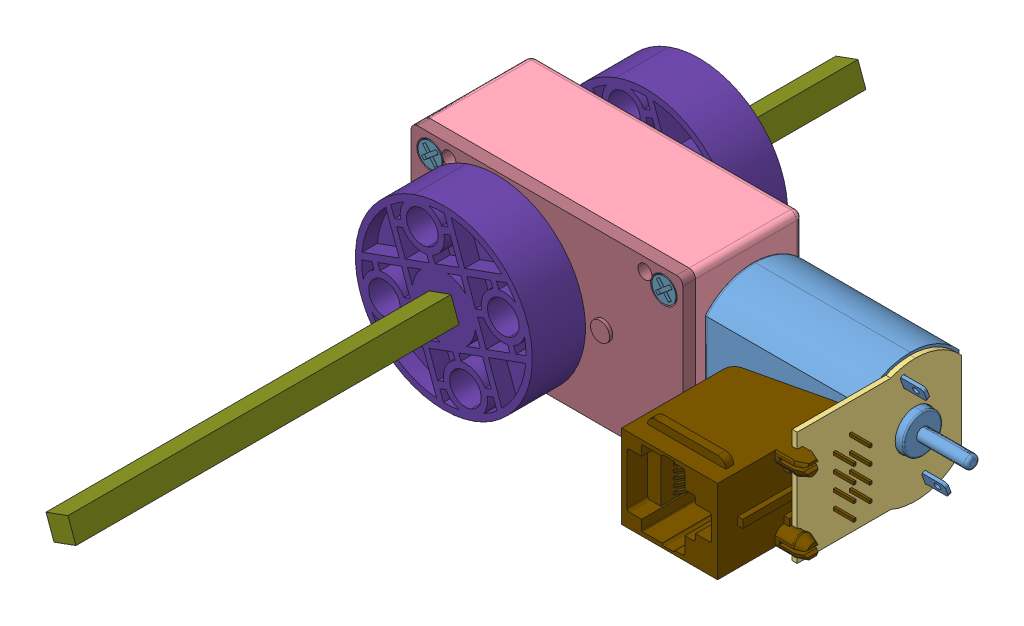
SolidWorks assembly MObeta, configuration Default. Lengths in mm.
Overall size (82.94 382.47 312.19).
32 component instances, 20 part files, 1 mates.
Components (placement in the parent):
- 玩具装配体1(1)(1)^MObeta-1: 玩具装配体1(1)(1)^MObeta [Default] at origin size (90 382.47 312.19) (virtual)
  - ____________ __^玩具装配体1(1)(1)_MObeta-1: ____________ __^玩具装配体1(1)(1)_MObeta [Default] at (8.1056 25.0507 27.7769) size (81.14 382.47 312.19) (virtual)
    - ________^____________ ___玩具装配体1(1)(1)_MObeta-1: ________^____________ ___玩具装配体1(1)(1)_MObeta [Default] at (-3.235 23.1684 17.3007) size (78 377.78 254.32) (virtual)
      - ________-1^_____________________ ___玩具装配体1(1)(1)_MObeta-1: ________-1^_____________________ ___玩具装配体1(1)(1)_MObeta [Default] at (79.0405 10.7038 66.7002) x (0 1 0) z (-1 0 0) size (376.94 254.32 40.6) (virtual)
        - 130____^________-1______________________ ___玩具装配体1(1)(1)_MObeta-1: 130____^________-1______________________ ___玩具装配体1(1)(1)_MObeta [Default] at (13.1972 32.2289 22.095) size (20.4 15.42 40.6) (virtual)
        - _________GearTrax^________-1______________________ ___玩具装配体1(1)(1)_MObeta-1: _________GearTrax^________-1______________________ ___玩具装配体1(1)(1)_MObeta [Default] at (13.1972 32.2289 60.0105) size (5.14 5.15 2.51) (virtual)
        - ______1^________-1______________________ ___玩具装配体1(1)(1)_MObeta-1: ______1^________-1______________________ ___玩具装配体1(1)(1)_MObeta [Default] at (13.1972 32.2289 21.695) x (-1 0 0) z (0 0 -1) size (376.94 254.32 0.8) (virtual)
      - ____^_____________________ ___玩具装配体1(1)(1)_MObeta-1: ____^_____________________ ___玩具装配体1(1)(1)_MObeta [Default] at (-11.0546 37.151 26.4713) size (43 26.5 17) (virtual)
      - ____-0^_____________________ ___玩具装配体1(1)(1)_MObeta-1: ____-0^_____________________ ___玩具装配体1(1)(1)_MObeta [Default] at (19.3454 23.901 27.4713) x (0.849881 -0.526974 0) z (0 0 1) size (2 2 17.3) (virtual)
    - __________^____________ ___玩具装配体1(1)(1)_MObeta-1: __________^____________ ___玩具装配体1(1)(1)_MObeta [Default] at (21.2756 42.8015 58.464) x (-0.874477 -0.485066 0) z (0 0 -1) size (21.33 21.33 6.2) (virtual)
      - Z13M0.6__6.2__^_______________________ ___玩具装配体1(1)(1)_MObeta-1: Z13M0.6__6.2__^_______________________ ___玩具装配体1(1)(1)_MObeta [Default] at (1173.14 3914.1005 3.992) size (9.48 9.54 6.2) (virtual)
      - _________GearTrax-1^_______________________ ___玩具装配体1(1)(1)_MObeta-1: _________GearTrax-1^_______________________ ___玩具装配体1(1)(1)_MObeta [Default] at (2.4466 6.2377 6.9147) x (-0.063071 0.998009 0) z (0 0 -1) size (20.1 20.11 1.51) (virtual)
    - ____22__38^____________ ___玩具装配体1(1)(1)_MObeta-1: ____22__38^____________ ___玩具装配体1(1)(1)_MObeta [Default] at (14.2004 56.9635 69.366) x (0.000452 -1 0) z (0 0 -1) size (23.9 23.96 6.2) (virtual)
      - Z38M0.6__2__^____22__38_____________ ___玩具装配体1(1)(1)_MObeta-1: Z38M0.6__2__^____22__38_____________ ___玩具装配体1(1)(1)_MObeta [Default] at (1346.5029 3922.186 16.084) size (23.9 23.96 2) (virtual)
      - Z22M0.6^____22__38_____________ ___玩具装配体1(1)(1)_MObeta-1: Z22M0.6^____22__38_____________ ___玩具装配体1(1)(1)_MObeta [Default] at (1192.4286 3849.0893 11.884) size (14.87 15 6.2) (virtual)
    - ____13__30^____________ ___玩具装配体1(1)(1)_MObeta-1: ____13__30^____________ ___玩具装配体1(1)(1)_MObeta [Default] at (10.1665 52.004 63.32) x (0.917069 0.398729 0) z (0 0 -1) size (18.53 18.6 5.5) (virtual)
      - Z13M0.6__5.5__^____13__30_____________ ___玩具装配体1(1)(1)_MObeta-1: Z13M0.6__5.5__^____13__30_____________ ___玩具装配体1(1)(1)_MObeta [Default] at (1248.1045 3738.5426 3.348) size (9.48 9.54 5.5) (virtual)
      - Z30M0.6^____13__30_____________ ___玩具装配体1(1)(1)_MObeta-1: Z30M0.6^____13__30_____________ ___玩具装配体1(1)(1)_MObeta [Default] at (1316.5243 3845.8896 6.848) size (18.53 18.6 2) (virtual)
    - Z38M0.6__18.9__^____________ ___玩具装配体1(1)(1)_MObeta-1: Z38M0.6__18.9__^____________ ___玩具装配体1(1)(1)_MObeta [Default] at (-156.8999 3954.1504 57.482) x (0.939862 0.341554 0) z (0 0 1) size (23.9 23.96 37.6) (virtual)
    - ____-2^____________ ___玩具装配体1(1)(1)_MObeta-1: ____-2^____________ ___玩具装配体1(1)(1)_MObeta [Default] at (-14.2896 33.8194 62.772) x (1 0 0) z (0 0 -1) size (43 26.5 18.5) (virtual)
    - ________-3^____________ ___玩具装配体1(1)(1)_MObeta-1: ________-3^____________ ___玩具装配体1(1)(1)_MObeta [Default] at (-11.2896 57.3194 61.772) x (0.644574 -0.764542 0) z (0 0 -1) size (3.8 3.8 14.01) (virtual)
    - ________-3^____________ ___玩具装配体1(1)(1)_MObeta-2: ________-3^____________ ___玩具装配体1(1)(1)_MObeta [Default] at (25.7104 57.3194 61.772) x (0.644574 -0.764542 0) z (0 0 -1) size (3.8 3.8 14.01) (virtual)
    - ________-3^____________ ___玩具装配体1(1)(1)_MObeta-3: ________-3^____________ ___玩具装配体1(1)(1)_MObeta [Default] at (25.7104 36.8194 61.772) x (0.644574 -0.764542 0) z (0 0 -1) size (3.8 3.8 14.01) (virtual)
    - ________-3^____________ ___玩具装配体1(1)(1)_MObeta-4: ________-3^____________ ___玩具装配体1(1)(1)_MObeta [Default] at (-11.2896 36.8194 61.772) x (0.644574 -0.764542 0) z (0 0 -1) size (3.8 3.8 14.01) (virtual)
    - ________-4^____________ ___玩具装配体1(1)(1)_MObeta-1: ________-4^____________ ___玩具装配体1(1)(1)_MObeta [Default] at (32.2104 53.2694 51.772) x (0 -0.340814 0.940131) z (-1 0 0) size (3.6 3.6 6.21) (virtual)
    - ________-4^____________ ___玩具装配体1(1)(1)_MObeta-2: ________-4^____________ ___玩具装配体1(1)(1)_MObeta [Default] at (32.2104 40.8694 51.772) x (0 -0.063636 0.997973) z (-1 0 0) size (3.6 3.6 6.21) (virtual)
    - ______^____________ ___玩具装配体1(1)(1)_MObeta-1: ______^____________ ___玩具装配体1(1)(1)_MObeta [Default] at (0.5104 47.0694 70.4668) x (0.939862 0.341554 0) z (0 0 1) size (3.7 3.7 125) (virtual)
    - ____-5^____________ ___玩具装配体1(1)(1)_MObeta-1: ____-5^____________ ___玩具装配体1(1)(1)_MObeta [Default] at (0.5104 47.0694 72.382) x (0 0 -1) z (0.939862 0.341554 0) size (8.4 28 28) (virtual)
    - ____-5^____________ ___玩具装配体1(1)(1)_MObeta-2: ____-5^____________ ___玩具装配体1(1)(1)_MObeta [Default] at (0.5104 47.0694 31.982) x (0 0 1) z (-0.939862 -0.341554 0) size (8.4 28 28) (virtual)
  - ____1^玩具装配体1(1)(1)_MObeta-1: ____1^玩具装配体1(1)(1)_MObeta [Default] at (28.616 72.1201 99.7488) x (1 0 0) z (0 0 -1) size (90 30 24) (hidden, virtual)
  - ____2^玩具装配体1(1)(1)_MObeta-1: ____2^玩具装配体1(1)(1)_MObeta [Default] at (28.616 72.1201 59.7488) size (90 30 20) (hidden, virtual)
- RJ45x1A-1: RJ45x1A [Default] at (53.513 72.1816 109.2399) x (0 1 0) z (0 0 1) size (15.75 20.02 20.6)
Mates (geometry in assembly coordinates):
- Coincident1: coincident anti-aligned: plane of 玩具装配体1(1)(1)^MObeta-1/____________ __^玩具装配体1(1)(1)_MObeta-1/________^____________ ___玩具装配体1(1)(1)_MObeta-1/________-1^_____________________ ___玩具装配体1(1)(1)_MObeta-1/______1^________-1______________________ ___玩具装配体1(1)(1)_MObeta-1 through (61.816 72.1201 79.5488) normal (-1 0 0); plane of RJ45x1A-1 through (61.816 79.9286 88.4119) normal (1 0 0)
